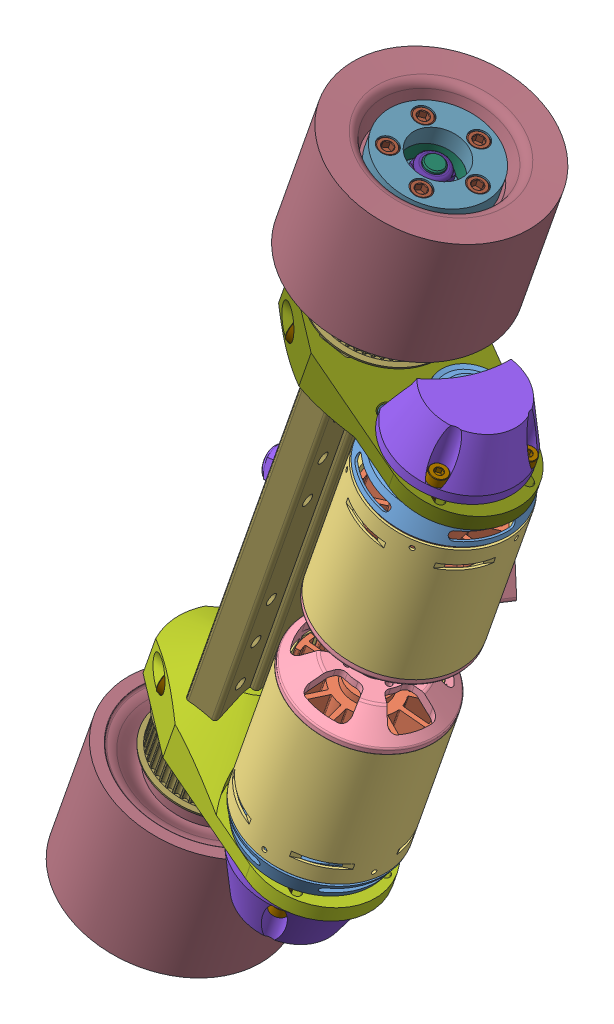
SolidWorks assembly MBS trucks pivot left, configuration Default. Lengths in mm.
Overall size (272 368.32 271.32).
89 component instances, 34 part files, 94 mates.
Components (placement in the parent):
- GPA26GT3150-A-N8-2: GPA26GT3150-A-N8 [Default] at (-15.9728 -53.3118 -54.0889) x (0.321551 0.946793 -0.013731) z (0.725283 -0.255593 -0.639248) size (20 28 28)
  - GPA26GT3150-A-N8_b-1: GPA26GT3150-A-N8_b [Default] at origin size (20 28 28)
  - SET-SCREW4-3-1: SET-SCREW4-3 [Default] at (10 5.4 0) x (0 -1 0) z (-1 0 0) size (3 4 4)
  - SET-SCREW4-3-2: SET-SCREW4-3 [Default] at (10 -2.2723 -3.2919) x (0 0.568065 0.822984) z (-1 0 0) size (3 4 4)
- Key20mm-2: Key20mm [Default] at (-13.4239 -54.1646 -53.2025) x (-0.725283 0.255593 0.639248) z (-0.608745 0.195591 -0.768878) size (3 20 3)
- MarkIITrucksCustomHanger pivot left-1: MarkIITrucksCustomHanger pivot left [Default] at (-31.1638 36.2817 -181.4556) x (-0.019038 0.999391 0.029249) z (0.838104 0 0.54551) size (362.13 183.87 195.64)
  - 50cal_baseplateEDIT-1: 50cal_baseplateEDIT [Default] at (40.8754 28.4427 48.4148) size (55.88 41.6 78.53)
  - BS_bushing-1: BS_bushing [Default] at (40.8754 74.2758 55.8381) x (0.903515 -0.328294 -0.275471) z (-0.428557 -0.692132 -0.580768) size (24.64 14.73 24.64)
  - BS_washer-1: BS_washer [Default] at (40.8754 63.8267 68.2909) x (0.781233 0.478195 0.401253) z (-0.624239 0.59846 0.502167) size (29.08 4.06 29.08)
  - kingpin-1: kingpin [Default] at (40.8754 51.905 82.4986) x (0.057682 0.764769 0.641717) z (0.998335 -0.044187 -0.037077) size (16.06 70.1 13.91)
  - kingpin-nut-1: kingpin-nut [90630A115] at (40.8754 87.1097 40.5433) x (0.976709 0.16437 0.137923) z (-0.214569 0.748202 0.627816) size (12.7 8.97 14.66)
  - Pivot_cup-1: Pivot_cup [Default] at (40.8754 44.9216 26.2393) x (-0.987309 0.102082 -0.121656) z (0.158811 0.63463 -0.756323) size (17.46 19.05 17.46)
  - RS_bushing-1: RS_bushing [Default] at (40.8754 76.7422 52.8988) x (0.999722 0.018072 0.015164) z (-0.023591 0.765831 0.642609) size (24.77 14.61 24.77)
  - washer-1: washer [Default] at (163.5053 59.317 96.5836) x (0.259291 0.957472 -0.126552) z (-0.223038 0.186855 0.956734) size (11 1 11)
  - BS_washer-2: BS_washer [Default] at (40.8754 87.1097 40.5433) x (-0.947616 0.244683 0.205314) z (0.319411 0.725916 0.609116) size (29.08 4.06 29.08)
  - washer-2: washer [Default] at (187.2325 53.7659 103.1992) x (-0.339774 -0.687707 0.641571) z (0.039134 -0.691901 -0.720931) size (11 1 11)
  - CustomHanger-1: CustomHanger [Default] at (40.8754 81.1126 56.6072) x (0.939693 -0.219846 0.262003) z (-0.34202 -0.604023 0.719846) size (253 93.96 18)
  - KegelWheelAssembly-1: KegelWheelAssembly [Default] at (219.4634 92.3673 64.2784) x (0.321079 0.830973 -0.454305) z (-0.11784 0.51103 0.851447) size (80 56 80)
    - Kegel 80mm longboard wheel-1: Kegel 80mm longboard wheel [Default] at (-60.1073 30.6906 17.2106) size (80 56 80)
    - 608-bearing-1: 608-bearing [6661K82] at (-60.1073 32.8534 17.2106) x (1 0 0) z (0 -1 0) size (22 22 7)
    - 608-bearing-2: 608-bearing [6661K82] at (-60.1073 15.6034 17.2106) x (-0.561464 0 0.827501) z (0 -1 0) size (22 22 7)
  - FPSSFJAD-D10-L64-T36-Q8-1: FPSSFJAD-D10-L64-T36-Q8 [Default] at (102.8951 73.4971 79.6845) x (0.939693 -0.219846 0.262003) z (-0.305917 -0.197698 0.931306) size (100 10 10)
  - SetScrew_SAE_10-32x.5in-1: SetScrew_SAE_10-32x.5in [92313A829] at (125.4477 77.0833 93.4091) x (0.758718 0.418725 -0.499016) z (0 0.766044 0.642788) size (4.96 4.83 13.07)
  - SetScrew_SAE_10-32x.5in-3: SetScrew_SAE_10-32x.5in [92313A829] at (125.446 59.3596 78.5344) x (0.758718 0.418725 -0.499016) z (0 -0.766044 -0.642788) size (4.96 4.83 13.07)
  - NylonLockNut_5.16-24-1: NylonLockNut_5.16-24 [97135A225] at (187.7024 53.656 103.3302) x (-0.176745 0.34369 0.922301) z (0.292812 0.912987 -0.284106) size (12.7 8.97 14.66)
  - KegelWheelAssembly-3: KegelWheelAssembly [Default] at (-99.1143 183.5416 5.8922) x (0.321079 0.830973 -0.454305) z (0.11784 -0.51103 -0.851447) size (80 56 80)
    - Kegel 80mm longboard wheel-1: Kegel 80mm longboard wheel [Default] at (-60.1073 30.6906 17.2106) size (80 56 80)
    - 608-bearing-1: 608-bearing [6661K82] at (-60.1073 32.8534 17.2106) x (1 0 0) z (0 -1 0) size (22 22 7)
    - 608-bearing-2: 608-bearing [6661K82] at (-60.1073 15.6034 17.2106) x (-0.561464 0 0.827501) z (0 -1 0) size (22 22 7)
  - FPSSFJAD-D10-L64-T36-Q8-3: FPSSFJAD-D10-L64-T36-Q8 [Default] at (-21.1443 102.5168 45.1001) x (-0.939693 0.219846 -0.262003) z (0.305917 0.197698 -0.931306) size (100 10 10)
  - NylonLockNut_5.16-24-3: NylonLockNut_5.16-24 [97135A225] at (-105.9516 122.3579 21.4544) x (0.176745 -0.34369 -0.922301) z (0.292812 0.912987 -0.284106) size (12.7 8.97 14.66)
  - SetScrew_SAE_10-32x.5in-7: SetScrew_SAE_10-32x.5in [92313A829] at (-43.6943 116.656 46.2483) x (-0.162487 0.634245 -0.755864) z (0 0.766044 0.642788) size (4.96 4.83 13.07)
  - SetScrew_SAE_10-32x.5in-8: SetScrew_SAE_10-32x.5in [92313A829] at (-43.6969 98.9306 31.3755) x (-0.162487 0.634245 -0.755864) z (0 -0.766044 -0.642788) size (4.96 4.83 13.07)
- 91274A172_COATED ALLOY STEEL SOCKET HEAD CAP SCREW-1: 91274A172_COATED ALLOY STEEL SOCKET HEAD CAP SCREW [91274A172] at (-39.3622 -9.9181 -56.7129) x (0.098878 -0.091252 0.990907) z (0.939117 -0.320732 -0.123247) size (9.53 9.53 32.48)
- 91274A172_COATED ALLOY STEEL SOCKET HEAD CAP SCREW-2: 91274A172_COATED ALLOY STEEL SOCKET HEAD CAP SCREW [91274A172] at (-43.3582 -9.0359 -89.4581) x (-0.342421 -0.903267 -0.258565) z (0.939117 -0.320732 -0.123247) size (9.53 9.53 32.48)
- 91274A172_COATED ALLOY STEEL SOCKET HEAD CAP SCREW-7: 91274A172_COATED ALLOY STEEL SOCKET HEAD CAP SCREW [91274A172] at (14.3369 148.1963 -59.006) x (-0.142744 -0.037907 -0.989034) z (0.939117 -0.320732 -0.123247) size (9.53 9.53 32.48)
- Turnigy6374-6: Turnigy6374 [Default] at (-10.4314 -14.5152 -52.975) x (0.287141 -0.111317 -0.951398) z (-0.902306 0.30198 -0.307657) size (83.4 113.65 83.4)
  - Stator-1: Stator [Default] at (3.7873 1.8989 -6.3731) size (58.75 9.22 58.75)
  - StatorPart2-1: StatorPart2 [Default] at (3.7873 -16.3511 -6.3731) size (50 66 50)
  - AxelHoldCover-1: AxelHoldCover [Default] at (3.7873 -60.8511 -6.3731) x (0.982235 0 -0.187653) z (0.187653 0 0.982235) size (59.15 61.5 59.15)
  - AxelHold-1: AxelHold [Default] at (3.7873 -60.8511 -6.3731) x (0.729158 0 0.684345) z (0.684345 0 -0.729158) size (59 18.5 59)
  - AxisCust-1: AxisCust [Default] at (3.7873 -73.3511 -6.3731) x (0.844889 0 -0.534942) z (0.534942 0 0.844889) size (8 113.65 8)
  - 90967A120_STAINLESS STEEL EXTERNAL RETAINING RING-1: 90967A120_STAINLESS STEEL EXTERNAL RETAINING RING [90967A120] at (3.7873 12.2489 -6.3731) x (0 -1 0) z (0 0 1) size (0.8 12.1 9.85)
  - 90967A120_STAINLESS STEEL EXTERNAL RETAINING RING-2: 90967A120_STAINLESS STEEL EXTERNAL RETAINING RING [90967A120] at (3.7873 -73.7511 -6.3731) x (0 -1 0) z (-0.841191 0 -0.540738) size (0.8 12.1 9.85)
- MotorMountLeft-3: MotorMountLeft [Default] at (-58.499 -16.8313 -71.1921) x (0.321551 0.946793 -0.013731) z (-0.287141 0.111317 0.951398) size (25.4 116.05 69.01)
- Belt Cap Wheel Side - Motor-2: Belt Cap Wheel Side - Motor [Default] at (-9.188 -33.3345 -54.3787) x (-0.287141 0.111317 0.951398) z (0.902306 -0.30198 0.307657) size (50.8 25 40.64)
- M4x16mm_BlackZincSteel-3: M4x16mm_BlackZincSteel [91274A119] at (13.174 -28.4024 -64.5577) x (0.938743 -0.320649 -0.126274) z (0.321551 0.946793 -0.013731) size (7 7 20.35)
- M4x16mm_BlackZincSteel-4: M4x16mm_BlackZincSteel [91274A119] at (4.2403 -24.939 -34.9571) x (0.938743 -0.320649 -0.126274) z (0.321551 0.946793 -0.013731) size (7 7 20.35)
- 92125A192_TYPE 18-8 SS FLAT-HEAD SOCKET CAP SCREW-9: 92125A192_TYPE 18-8 SS FLAT-HEAD SOCKET CAP SCREW [92125A192] at (-18.6935 -30.1791 -73.9677) x (-0.475481 0.17399 0.862349) z (-0.321551 -0.946793 0.013731) size (8 8 12.4)
- 92125A192_TYPE 18-8 SS FLAT-HEAD SOCKET CAP SCREW-10: 92125A192_TYPE 18-8 SS FLAT-HEAD SOCKET CAP SCREW [92125A192] at (-27.6272 -26.7157 -44.3671) x (0.938569 -0.320609 -0.127663) z (-0.321551 -0.946793 0.013731) size (8 8 12.4)
- 91251A355_BLACK-OXIDE ALLOY STEEL SOCKET HEAD CAP SCREW-11: 91251A355_BLACK-OXIDE ALLOY STEEL SOCKET HEAD CAP SCREW [91251A355] at (-57.9016 -22.5836 -86.7863) x (0.946372 -0.32086 0.0378) z (0.321551 0.946793 -0.013731) size (7.92 7.92 68.91)
- GPA50GT3150-A-H26_b-1: GPA50GT3150-A-H26_b [Default] at (-58.901 -18.0147 -71.1749) x (-0.321551 -0.946793 0.013731) z (0.936494 -0.315843 0.152386) size (20 51 51)
- Wheel Spacer 2-3: Wheel Spacer 2 [Default] at (-71.5742 -55.3305 -70.6337) x (-0.156301 0.038769 -0.986948) z (0.933903 -0.3195 -0.160451) size (44 14.02 44)
- Wheel Spacer Alum-3: Wheel Spacer Alum [Default] at (-71.5742 -55.3305 -70.6337) x (-0.156301 0.038769 -0.986948) z (0.933903 -0.3195 -0.160451) size (44 7.62 44)
- 91251A355_BLACK-OXIDE ALLOY STEEL SOCKET HEAD CAP SCREW-12: 91251A355_BLACK-OXIDE ALLOY STEEL SOCKET HEAD CAP SCREW [91251A355] at (-73.5512 -17.145 -78.2602) x (0.322292 -0.12307 -0.938606) z (0.321551 0.946793 -0.013731) size (7.92 7.92 68.91)
- 91251A355_BLACK-OXIDE ALLOY STEEL SOCKET HEAD CAP SCREW-13: 91251A355_BLACK-OXIDE ALLOY STEEL SOCKET HEAD CAP SCREW [91251A355] at (-70.6389 -17.8674 -59.8706) x (-0.747185 0.244798 -0.61789) z (0.321551 0.946793 -0.013731) size (7.92 7.92 68.91)
- 91251A355_BLACK-OXIDE ALLOY STEEL SOCKET HEAD CAP SCREW-14: 91251A355_BLACK-OXIDE ALLOY STEEL SOCKET HEAD CAP SCREW [91251A355] at (-53.1894 -23.7524 -57.0313) x (-0.784077 0.274364 0.556729) z (0.321551 0.946793 -0.013731) size (7.92 7.92 68.91)
- 91251A355_BLACK-OXIDE ALLOY STEEL SOCKET HEAD CAP SCREW-15: 91251A355_BLACK-OXIDE ALLOY STEEL SOCKET HEAD CAP SCREW [91251A355] at (-45.3173 -26.6672 -73.666) x (0.262598 -0.075232 0.961968) z (0.321551 0.946793 -0.013731) size (7.92 7.92 68.91)
- Wheel Spacer-3: Wheel Spacer [Default] at (-71.5742 -55.3305 -70.6337) x (0.139941 -0.061859 -0.988226) z (0.936494 -0.315843 0.152386) size (44 7.02 44)
- 91274A172_COATED ALLOY STEEL SOCKET HEAD CAP SCREW-8: 91274A172_COATED ALLOY STEEL SOCKET HEAD CAP SCREW [91274A172] at (14.3369 148.1963 -59.006) x (-0.142744 -0.037907 -0.989034) z (0.939117 -0.320732 -0.123247) size (9.53 9.53 32.48)
- 91274A172_COATED ALLOY STEEL SOCKET HEAD CAP SCREW-9: 91274A172_COATED ALLOY STEEL SOCKET HEAD CAP SCREW [91274A172] at (10.3408 149.0785 -91.7513) x (-0.27609 -0.917912 0.284977) z (0.939117 -0.320732 -0.123247) size (9.53 9.53 32.48)
- Turnigy6374-7: Turnigy6374 [Default] at (51.6181 130.4737 -51.2122) x (0.287141 -0.111317 -0.951398) z (0.902306 -0.30198 0.307657) size (83.4 113.65 83.4)
  - Stator-1: Stator [Default] at (3.7873 1.8989 -6.3731) size (58.75 9.22 58.75)
  - StatorPart2-1: StatorPart2 [Default] at (3.7873 -16.3511 -6.3731) size (50 66 50)
  - AxelHoldCover-1: AxelHoldCover [Default] at (3.7873 -60.8511 -6.3731) x (0.982235 0 -0.187653) z (0.187653 0 0.982235) size (59.15 61.5 59.15)
  - AxelHold-1: AxelHold [Default] at (3.7873 -60.8511 -6.3731) x (0.729158 0 0.684345) z (0.684345 0 -0.729158) size (59 18.5 59)
  - AxisCust-1: AxisCust [Default] at (3.7873 -73.3511 -6.3731) x (0.844889 0 -0.534942) z (0.534942 0 0.844889) size (8 113.65 8)
  - 90967A120_STAINLESS STEEL EXTERNAL RETAINING RING-1: 90967A120_STAINLESS STEEL EXTERNAL RETAINING RING [90967A120] at (3.7873 12.2489 -6.3731) x (0 -1 0) z (0 0 1) size (0.8 12.1 9.85)
  - 90967A120_STAINLESS STEEL EXTERNAL RETAINING RING-2: 90967A120_STAINLESS STEEL EXTERNAL RETAINING RING [90967A120] at (3.7873 -73.7511 -6.3731) x (0 -1 0) z (-0.841191 0 -0.540738) size (0.8 12.1 9.85)
- Belt Cap Wheel Side - Motor-3: Belt Cap Wheel Side - Motor [Default] at (52.5497 148.4497 -57.0151) x (0.287141 -0.111317 -0.951398) z (0.902306 -0.30198 0.307657) size (50.8 25 40.64)
- M4x16mm_BlackZincSteel-5: M4x16mm_BlackZincSteel [91274A119] at (67.1946 130.6588 -66.8646) x (0.938743 -0.320649 -0.126274) z (-0.321551 -0.946793 0.013731) size (7 7 20.35)
- M4x16mm_BlackZincSteel-6: M4x16mm_BlackZincSteel [91274A119] at (58.2608 134.1222 -37.264) x (0.938743 -0.320649 -0.126274) z (-0.321551 -0.946793 0.013731) size (7 7 20.35)
- 92125A192_TYPE 18-8 SS FLAT-HEAD SOCKET CAP SCREW-11: 92125A192_TYPE 18-8 SS FLAT-HEAD SOCKET CAP SCREW [92125A192] at (42.9157 151.2264 -76.5987) x (0.475481 -0.17399 -0.862349) z (0.321551 0.946793 -0.013731) size (8 8 12.4)
- 92125A192_TYPE 18-8 SS FLAT-HEAD SOCKET CAP SCREW-12: 92125A192_TYPE 18-8 SS FLAT-HEAD SOCKET CAP SCREW [92125A192] at (33.982 154.6898 -46.9981) x (0.938569 -0.320609 -0.127663) z (0.321551 0.946793 -0.013731) size (8 8 12.4)
- 91251A355_BLACK-OXIDE ALLOY STEEL SOCKET HEAD CAP SCREW-16: 91251A355_BLACK-OXIDE ALLOY STEEL SOCKET HEAD CAP SCREW [91251A355] at (7.0774 168.7443 -89.5611) x (0.946372 -0.32086 0.0378) z (-0.321551 -0.946793 0.013731) size (7.92 7.92 68.91)
- GPA50GT3150-A-H26_b-2: GPA50GT3150-A-H26_b [Default] at (3.6407 166.1364 -73.8457) x (0.321551 0.946793 -0.013731) z (-0.936494 0.315843 -0.152386) size (20 51 51)
- Wheel Spacer 2-4: Wheel Spacer 2 [Default] at (16.3139 203.4522 -74.3869) x (0.156301 -0.038769 0.986948) z (0.933903 -0.3195 -0.160451) size (44 14.02 44)
- Wheel Spacer Alum-4: Wheel Spacer Alum [Default] at (16.3139 203.4522 -74.3869) x (0.156301 -0.038769 0.986948) z (0.933903 -0.3195 -0.160451) size (44 7.62 44)
- Wheel Spacer-4: Wheel Spacer [Default] at (16.3139 203.4522 -74.3869) x (0.139941 -0.061859 -0.988226) z (-0.936494 0.315843 -0.152386) size (44 7.02 44)
- GPA26GT3150-A-N8-3: GPA26GT3150-A-N8 [Default] at (52.9034 149.4912 -57.0302) x (0.321551 0.946793 -0.013731) z (0.725283 -0.255593 -0.639248) size (20 28 28)
  - GPA26GT3150-A-N8_b-1: GPA26GT3150-A-N8_b [Default] at origin size (20 28 28)
  - SET-SCREW4-3-1: SET-SCREW4-3 [Default] at (10 5.4 0) x (0 -1 0) z (-1 0 0) size (3 4 4)
  - SET-SCREW4-3-2: SET-SCREW4-3 [Default] at (10 -2.2723 -3.2919) x (0 0.568065 0.822984) z (-1 0 0) size (3 4 4)
- Key20mm-3: Key20mm [Default] at (63.7096 166.9875 -54.1118) x (-0.725283 0.255593 0.639248) z (0.608745 -0.195591 0.768878) size (3 20 3)
- MotorMountRight-2: MotorMountRight [Default] at (3.2387 164.9529 -73.8285) x (0.321551 0.946793 -0.013731) z (-0.287141 0.111317 0.951398) size (25.4 116.05 69.01)
- 91251A355_BLACK-OXIDE ALLOY STEEL SOCKET HEAD CAP SCREW-17: 91251A355_BLACK-OXIDE ALLOY STEEL SOCKET HEAD CAP SCREW [91251A355] at (19.6617 164.6607 -76.4409) x (-0.262598 0.075232 -0.961968) z (-0.321551 -0.946793 0.013731) size (7.92 7.92 68.91)
- 91251A355_BLACK-OXIDE ALLOY STEEL SOCKET HEAD CAP SCREW-18: 91251A355_BLACK-OXIDE ALLOY STEEL SOCKET HEAD CAP SCREW [91251A355] at (11.7897 167.5755 -59.8061) x (-0.784077 0.274364 0.556729) z (-0.321551 -0.946793 0.013731) size (7.92 7.92 68.91)
- 91251A355_BLACK-OXIDE ALLOY STEEL SOCKET HEAD CAP SCREW-19: 91251A355_BLACK-OXIDE ALLOY STEEL SOCKET HEAD CAP SCREW [91251A355] at (-5.6598 173.4605 -62.6455) x (-0.747185 0.244798 -0.61789) z (-0.321551 -0.946793 0.013731) size (7.92 7.92 68.91)
- 91251A355_BLACK-OXIDE ALLOY STEEL SOCKET HEAD CAP SCREW-20: 91251A355_BLACK-OXIDE ALLOY STEEL SOCKET HEAD CAP SCREW [91251A355] at (-8.5722 174.1829 -81.0351) x (-0.322292 0.12307 0.938606) z (-0.321551 -0.946793 0.013731) size (7.92 7.92 68.91)
Mates (geometry in assembly coordinates):
- Concentric1: concentric anti-aligned: cylinder of ? through (0 89.5 0) axis (0 -1 0) radius 6; cylinder of ? through (0 92.55 0) axis (0 1 0) radius 6
- Concentric2: concentric anti-aligned: cylinder of ? through (0 -26.5 0) axis (0 1 0) radius 4; cylinder of GPA26GT3150-A-N8-2/GPA26GT3150-A-N8_b-1 through (0 -6.5 0) axis (0 -1 0) radius 4
- Coincident1: coincident aligned: plane of ? through (0 -26.5 0) normal (0 -1 0); plane of GPA26GT3150-A-N8-2/GPA26GT3150-A-N8_b-1 through (0 -26.5 0) normal (0 -1 0)
- Coincident7: coincident anti-aligned: line of ? through (-1.5 -26.5 -2.5) axis (0 0 -1); line of GPA26GT3150-A-N8-2/GPA26GT3150-A-N8_b-1 through (-1.5 -26.5 -5.4) axis (0 0 1)
- Coincident8: coincident aligned: plane of GPA26GT3150-A-N8-2/GPA26GT3150-A-N8_b-1 through (-15.9728 -53.3118 -54.0889) normal (-0.321551 -0.946793 0.013731); plane of Key20mm-2 through (-13.4239 -54.1646 -53.2025) normal (-0.321551 -0.946793 0.013731)
- Coincident9: coincident anti-aligned: plane of ? through (1.5 -6.5 -2.5) normal (0 0 -1); plane of Key20mm-2 through (-1.5 -6.5 -2.5) normal (0 0 1)
- Coincident10: coincident anti-aligned: plane of GPA26GT3150-A-N8-2/GPA26GT3150-A-N8_b-1 through (-5.1666 -35.8155 -51.1705) normal (-0.725283 0.255593 0.639248); plane of Key20mm-2 through (-6.9928 -35.2288 -53.4771) normal (0.725283 -0.255593 -0.639248)
- Concentric5: concentric anti-aligned: cylinder of MarkIITrucksCustomHanger pivot left-1/CustomHanger-1 through (-77.4086 -5.45 -20.7444) axis (0 -1 0) radius 9; cylinder of ? through (-77.4086 -27.45 -20.7444) axis (0 1 0) radius 11
- Coincident15: coincident anti-aligned: plane of ? through (-77.2299 -26.5 -21.3999) normal (0 1 0); plane of ? through (-51.5162 -26.5 -25.2476) normal (0 -1 0)
- Coincident28: coincident anti-aligned: plane of MarkIITrucksCustomHanger pivot left-1/CustomHanger-1; plane of ? through (-34.0921 -14.7886 -63.0299) normal (-0.017088 0 -0.999854)
- Coincident37: coincident aligned: plane of ? through (-44.2534 59.243 -27.1128) normal (-0.40707 0 0.913397); plane of ? through (38.0802 32.893 9.5804) normal (-0.40707 0 0.913397)
- Coincident38: coincident anti-aligned: plane of ? through (-30.006 52.893 -59.0817) normal (0 -1 0); plane of ? through (52.3276 52.893 -22.3885) normal (0 1 0)
- Coincident40: coincident anti-aligned: plane of ? through (0 0 0) normal (0 -1 0); plane of ? through (-73.3266 0 -32.3363) normal (0 1 0)
- Concentric12: concentric aligned: cylinder of ? through (0 -26.5 0) axis (0 1 0) radius 4; cylinder of ? through (0 -6.35 0) axis (0 1 0) radius 6
- Coincident41: coincident anti-aligned: plane of ?; plane of ? through (-51.7284 -27.45 -24.8099) normal (0 -1 0)
- Concentric17: concentric aligned: cylinder of MarkIITrucksCustomHanger pivot left-1/CustomHanger-1 through (-34.2459 -20.2386 -72.0286) axis (0 -1 0) radius 9; cylinder of ? through (-34.2459 -22.2386 -72.0286) axis (0 -1 0) radius 10
- Coincident43: coincident anti-aligned: plane of ?; plane of ? through (-34.2459 -42.2386 -72.0286) normal (0 -1 0)
- Concentric18: concentric anti-aligned: cylinder of ? through (-93.4436 208.55 -19.2392) axis (0 -1 0) radius 2.54; cylinder of ? through (-93.4436 193.63 -19.2392) axis (0 1 0) radius 2.413
- Coincident45: coincident anti-aligned: plane of ? through (-93.4436 193.63 -19.2392) normal (0 -1 0); plane of ? through (-93.4436 193.63 -19.2392) normal (0 1 0)
- Concentric19: concentric: cylinder of ? through (-93.4436 208.55 -19.2392) axis (0 -1 0) radius 2.54; cylinder of ? through (-93.4436 193.63 -19.2392) axis (0 1 0) radius 2.413
- Coincident47: coincident anti-aligned: plane of ? through (-93.4436 193.63 -19.2392) normal (0 -1 0); plane of ? through (-93.4436 193.63 -19.2392) normal (0 1 0)
- Coincident48: coincident anti-aligned: plane of ?; plane of ? through (-43.0816 192.3928 -91.4524) normal (-0.019038 0.999391 0.029249)
- Concentric28: concentric anti-aligned: cylinder of ? through (-15.3407 192.0809 -62.7407) axis (-0.019038 0.999391 0.029249) radius 2.9; cylinder of ? through (-16.2508 239.8547 -61.3425) axis (0.019038 -0.999391 -0.029249) radius 2.413
- Coincident56: coincident anti-aligned: plane of GPA26GT3150-A-N8-2/GPA26GT3150-A-N8_b-1 through (-7.3425 -35.0487 -49.2527) normal (-0.608745 0.195591 -0.768878); plane of Key20mm-2 through (-5.1666 -35.8155 -51.1705) normal (0.608745 -0.195591 0.768878)
- Coincident58: coincident aligned: plane of GPA26GT3150-A-N8-2/GPA26GT3150-A-N8_b-1; plane of ? through (-22.9313 -22.2386 -48.6196) normal (0 1 0)
- Concentric38: concentric aligned: cylinder of MarkIITrucksCustomHanger pivot left-1/CustomHanger-1 through (-41.8828 -7.7386 -55.3957) axis (0.999854 0 -0.017088) radius 2.3813; cylinder of ? through (-80.4696 -7.7386 -54.7362) axis (0.999854 0 -0.017088) radius 5
- Concentric40: concentric aligned: cylinder of ? through (-81.0335 -7.7386 -87.7314) axis (0.999854 0 -0.017088) radius 5; cylinder of 91274A172_COATED ALLOY STEEL SOCKET HEAD CAP SCREW-2 through (-52.2253 -7.7386 -88.2237) axis (0.999854 0 -0.017088) radius 4.7625
- Concentric41: concentric aligned: cylinder of ? through (-80.4696 -7.7386 -54.7362) axis (0.999854 0 -0.017088) radius 5; cylinder of 91274A172_COATED ALLOY STEEL SOCKET HEAD CAP SCREW-1 through (-51.6614 -7.7386 -55.2286) axis (0.999854 0 -0.017088) radius 4.7625
- Coincident61: coincident anti-aligned: plane of ? through (-45.3123 -7.7386 -55.3371) normal (-0.999854 0 0.017088); plane of 91274A172_COATED ALLOY STEEL SOCKET HEAD CAP SCREW-1 through (-45.3123 -7.7386 -55.3371) normal (0.999854 0 -0.017088)
- Coincident62: coincident anti-aligned: plane of ? through (-45.8762 -7.7386 -88.3322) normal (-0.999854 0 0.017088); plane of 91274A172_COATED ALLOY STEEL SOCKET HEAD CAP SCREW-2 through (-45.8762 -7.7386 -88.3322) normal (0.999854 0 -0.017088)
- Coincident65: coincident anti-aligned: plane of MarkIITrucksCustomHanger pivot left-1/CustomHanger-1; plane of ? through (-40.595 4.2614 -71.9201) normal (0.999854 0 -0.017088)
- Coincident68: coincident anti-aligned: plane of ? through (-34.2459 -14.7886 -72.0286) normal (0 1 0); plane of Turnigy6374-6/Stator-1 through (52.6547 -14.7886 -33.3) normal (0 -1 0)
- Concentric46: concentric anti-aligned: cylinder of GPA26GT3150-A-N8-2/GPA26GT3150-A-N8_b-1 through (-9.5418 -34.3759 -54.3635) axis (-0.321551 -0.946793 0.013731) radius 4; cylinder of Turnigy6374-6/AxisCust-1 through (-15.6995 -52.507 -54.1006) axis (0.321551 0.946793 -0.013731) radius 4
- Coincident70: coincident anti-aligned: plane of Key20mm-2 through (-6.9928 -35.2288 -53.4771) normal (0.725283 -0.255593 -0.639248); plane of Turnigy6374-6/AxisCust-1 through (-5.1057 -35.8351 -51.0936) normal (-0.725283 0.255593 0.639248)
- Concentric55: concentric aligned: cylinder of 91274A172_COATED ALLOY STEEL SOCKET HEAD CAP SCREW-1 through (-51.6614 -7.7386 -55.2286) axis (0.999854 0 -0.017088) radius 4.7625; cylinder of ? through (-80.4696 -7.7386 -54.7362) axis (0.999854 0 -0.017088) radius 3.175
- Coincident75: coincident anti-aligned: plane of 91274A172_COATED ALLOY STEEL SOCKET HEAD CAP SCREW-1; plane of ? through (-45.3123 -7.7386 -55.3371) normal (-0.999854 0 0.017088)
- Coincident76: coincident anti-aligned: plane of MarkIITrucksCustomHanger pivot left-1/CustomHanger-1; plane of ? through (-40.595 4.2614 -71.9201) normal (0.999854 0 -0.017088)
- Coincident77: coincident anti-aligned: plane of MarkIITrucksCustomHanger pivot left-1/CustomHanger-1; plane of ? through (-34.0921 -14.7886 -63.0299) normal (-0.017088 0 -0.999854)
- Concentric56: concentric aligned: cylinder of 91274A172_COATED ALLOY STEEL SOCKET HEAD CAP SCREW-2 through (-54.3819 -7.7386 -88.1869) axis (0.999854 0 -0.017088) radius 4.7625; cylinder of ? through (-81.0335 -7.7386 -87.7314) axis (0.999854 0 -0.017088) radius 5
- Concentric57: concentric aligned: cylinder of MarkIITrucksCustomHanger pivot left-1/CustomHanger-1 through (-41.8828 -7.7386 -55.3957) axis (0.999854 0 -0.017088) radius 2.3813; cylinder of ? through (-80.4696 -7.7386 -54.7362) axis (0.999854 0 -0.017088) radius 5
- Concentric58: concentric aligned: cylinder of 91274A172_COATED ALLOY STEEL SOCKET HEAD CAP SCREW-7 through (-51.6614 159.2614 -55.2286) axis (0.999854 0 -0.017088) radius 4.7625; cylinder of ? through (-80.4696 159.2614 -54.7362) axis (0.999854 0 -0.017088) radius 5
- Coincident78: coincident anti-aligned: plane of 91274A172_COATED ALLOY STEEL SOCKET HEAD CAP SCREW-7; plane of ? through (-45.3123 159.2614 -55.3371) normal (-0.999854 0 0.017088)
- Concentric59: concentric aligned: cylinder of 91274A172_COATED ALLOY STEEL SOCKET HEAD CAP SCREW-8 through (-52.2253 159.2614 -88.2237) axis (0.999854 0 -0.017088) radius 4.7625; cylinder of ? through (-81.0335 159.2614 -87.7314) axis (0.999854 0 -0.017088) radius 5
- Coincident79: coincident anti-aligned: plane of MarkIITrucksCustomHanger pivot left-1/CustomHanger-1; plane of ? through (-43.2446 -0.6886 -71.8748) normal (0.999854 0 -0.017088)
- Concentric60: concentric anti-aligned: cylinder of 91274A172_COATED ALLOY STEEL SOCKET HEAD CAP SCREW-2 through (-52.2253 -7.7386 -88.2237) axis (0.999854 0 -0.017088) radius 4.7625; circle of ?
- Coincident80: coincident anti-aligned: plane of 91274A172_COATED ALLOY STEEL SOCKET HEAD CAP SCREW-2; plane of ? through (-45.8762 -7.7386 -88.3322) normal (-0.999854 0 0.017088)
- Concentric61: concentric aligned: cylinder of MarkIITrucksCustomHanger pivot left-1/CustomHanger-1 through (-63.9155 -2.015 -86.7603) axis (0.939117 -0.320732 -0.123247) radius 2.3813; cylinder of 91274A172_COATED ALLOY STEEL SOCKET HEAD CAP SCREW-2 through (-73.1752 1.1474 -85.5451) axis (0.939117 -0.320732 -0.123247) radius 4.7625
- Concentric62: concentric aligned: cylinder of MarkIITrucksCustomHanger pivot left-1/CustomHanger-1 through (-41.8828 -7.7386 -55.3957) axis (0.999854 0 -0.017088) radius 2.3813; cylinder of ? through (-80.4696 -7.7386 -54.7362) axis (0.999854 0 -0.017088) radius 3.175
- Concentric63: concentric: cylinder of 91274A172_COATED ALLOY STEEL SOCKET HEAD CAP SCREW-1 through (-51.6614 -7.7386 -55.2286) axis (0.999854 0 -0.017088) radius 4.7625; cylinder of ? through (-80.4696 -7.7386 -54.7362) axis (0.999854 0 -0.017088) radius 5
- Coincident81: coincident anti-aligned: plane of 91274A172_COATED ALLOY STEEL SOCKET HEAD CAP SCREW-1; plane of ? through (-45.3123 -7.7386 -55.3371) normal (-0.999854 0 0.017088)
- Coincident86: coincident aligned: plane of GPA26GT3150-A-N8-2/GPA26GT3150-A-N8_b-1 through (-15.9728 -53.3118 -54.0889) normal (-0.321551 -0.946793 0.013731); plane of Turnigy6374-6/AxisCust-1 through (-15.9728 -53.3118 -54.0889) normal (-0.321551 -0.946793 0.013731)
- Coincident87: coincident anti-aligned: plane of MarkIITrucksCustomHanger pivot left-1/CustomHanger-1; plane of ? through (-33.8358 147.2614 -48.0321) normal (-0.017088 0 -0.999854)
- Concentric72: concentric aligned: cylinder of MarkIITrucksCustomHanger pivot left-1/CustomHanger-1 through (-6.2204 155.2171 -56.3081) axis (0.939117 -0.320732 -0.123247) radius 2.3813; cylinder of 91274A172_COATED ALLOY STEEL SOCKET HEAD CAP SCREW-7 through (-15.4801 158.3795 -55.0929) axis (0.939117 -0.320732 -0.123247) radius 4.7625
- Concentric73: concentric aligned: cylinder of 91274A172_COATED ALLOY STEEL SOCKET HEAD CAP SCREW-1 through (-69.1791 0.2651 -52.7998) axis (0.939117 -0.320732 -0.123247) radius 4.7625; cylinder of MotorMountLeft-3 through (-123.8058 18.9215 -45.6308) axis (0.939117 -0.320732 -0.123247) radius 5
- Concentric74: concentric aligned: cylinder of 91274A172_COATED ALLOY STEEL SOCKET HEAD CAP SCREW-2 through (-73.1752 1.1474 -85.5451) axis (0.939117 -0.320732 -0.123247) radius 4.7625; cylinder of MotorMountLeft-3 through (-127.8019 19.8037 -78.376) axis (0.939117 -0.320732 -0.123247) radius 5
- Coincident99: coincident anti-aligned: plane of MarkIITrucksCustomHanger pivot left-1/CustomHanger-1 through (4.6296 200.2711 -82.1167) normal (-0.939117 0.320732 0.123247); plane of MotorMountLeft-3 through (-64.9093 -7.9325 -70.1701) normal (0.939117 -0.320732 -0.123247)
- Coincident100: coincident anti-aligned: plane of 91274A172_COATED ALLOY STEEL SOCKET HEAD CAP SCREW-1 through (-63.2157 -1.7715 -53.5824) normal (0.939117 -0.320732 -0.123247); plane of MotorMountLeft-3 through (-63.2157 -1.7715 -53.5824) normal (-0.939117 0.320732 0.123247)
- Coincident101: coincident anti-aligned: plane of 91274A172_COATED ALLOY STEEL SOCKET HEAD CAP SCREW-2 through (-67.2118 -0.8893 -86.3277) normal (0.939117 -0.320732 -0.123247); plane of MotorMountLeft-3 through (-67.2118 -0.8893 -86.3277) normal (-0.939117 0.320732 0.123247)
- Coincident108: coincident anti-aligned: plane of Turnigy6374-6/Stator-1 through (-7.1462 -27.3223 -54.4658) normal (-0.321551 -0.946793 0.013731); plane of MotorMountLeft-3 through (-56.4572 -10.8191 -71.2793) normal (0.321551 0.946793 -0.013731)
- Concentric92: concentric aligned: cylinder of Belt Cap Wheel Side - Motor-2 through (0.9551 -64.3805 -64.0359) axis (0.321551 0.946793 -0.013731) radius 4; cylinder of M4x16mm_BlackZincSteel-3 through (6.743 -47.3382 -64.2831) axis (0.321551 0.946793 -0.013731) radius 3.5
- Concentric93: concentric aligned: cylinder of Belt Cap Wheel Side - Motor-2 through (-7.9786 -60.9171 -34.4353) axis (0.321551 0.946793 -0.013731) radius 4; cylinder of M4x16mm_BlackZincSteel-4 through (-2.1907 -43.8748 -34.6825) axis (0.321551 0.946793 -0.013731) radius 3.5
- Coincident121: coincident anti-aligned: plane of Belt Cap Wheel Side - Motor-2 through (8.0292 -43.551 -64.338) normal (-0.321551 -0.946793 0.013731); plane of M4x16mm_BlackZincSteel-3 through (8.0292 -43.551 -64.338) normal (0.321551 0.946793 -0.013731)
- Coincident122: coincident anti-aligned: plane of Belt Cap Wheel Side - Motor-2 through (-0.9045 -40.0877 -34.7374) normal (-0.321551 -0.946793 0.013731); plane of M4x16mm_BlackZincSteel-4 through (-0.9045 -40.0877 -34.7374) normal (0.321551 0.946793 -0.013731)
- Coincident123: coincident anti-aligned: plane of MotorMountLeft-3 through (-58.499 -16.8313 -71.1921) normal (-0.321551 -0.946793 0.013731); plane of Belt Cap Wheel Side - Motor-2 through (-9.188 -33.3345 -54.3787) normal (0.321551 0.946793 -0.013731)
- Tangent4: tangent anti-aligned: plane of MotorMountLeft-3; cone of ? through (71.8505 -7.1277 -46.5804) axis (-0.019038 0.999391 0.029249)
- Tangent5: tangent anti-aligned: plane of MotorMountLeft-3; cone of ? through (89.6321 -19.6632 -21.2486) axis (-0.019038 0.999391 0.029249)
- Tangent9: tangent anti-aligned: plane of MotorMountLeft-3; cone of ? through (89.6321 -19.6632 -21.2486) axis (-0.019038 0.999391 0.029249)
- Tangent10: tangent: plane of MotorMountLeft-3; curve of ?
- Concentric105: concentric anti-aligned: cylinder of Turnigy6374-6/Stator-1 through (89.3833 -6.6015 -20.8663) axis (0.019038 -0.999391 -0.029249) radius 1.8559; circle of ?
- Concentric106: concentric anti-aligned: cylinder of Turnigy6374-6/Stator-1 through (71.8325 -6.1841 -46.5528) axis (0.019038 -0.999391 -0.029249) radius 1.8559; circle of ?
- Concentric107: concentric anti-aligned: cylinder of Turnigy6374-6/Stator-1 through (14.3218 -25.0226 -64.6067) axis (-0.321551 -0.946793 0.013731) radius 1.8559; circle of M4x16mm_BlackZincSteel-3
- Concentric108: concentric anti-aligned: cylinder of Turnigy6374-6/Stator-1 through (5.3881 -21.5593 -35.0061) axis (-0.321551 -0.946793 0.013731) radius 1.8559; cylinder of M4x16mm_BlackZincSteel-4 through (-2.1907 -43.8748 -34.6825) axis (0.321551 0.946793 -0.013731) radius 3.5
- Tangent18: tangent anti-aligned: plane of MotorMountLeft-3 through (-52.7401 -19.0639 -90.2737) normal (-0.43041 -0.59077 0.68245); cone of 92125A192_TYPE 18-8 SS FLAT-HEAD SOCKET CAP SCREW-9 through (-17.9539 -28.0015 -73.9993) axis (0.321551 0.946793 -0.013731)
- Tangent19: tangent anti-aligned: plane of MotorMountLeft-3 through (-62.7363 -12.5099 -54.5233) normal (-0.024332 -0.748197 -0.663031); cone of 92125A192_TYPE 18-8 SS FLAT-HEAD SOCKET CAP SCREW-10 through (-26.8876 -24.5381 -44.3987) axis (0.321551 0.946793 -0.013731)
- Concentric109: concentric anti-aligned: cylinder of Turnigy6374-6/Stator-1 through (-22.6851 -12.1638 -44.5782) axis (-0.321551 -0.946793 0.013731) radius 1.8559; circle of 92125A192_TYPE 18-8 SS FLAT-HEAD SOCKET CAP SCREW-10
- Concentric110: concentric anti-aligned: cylinder of Turnigy6374-6/Stator-1 through (-13.7513 -15.6272 -74.1787) axis (-0.321551 -0.946793 0.013731) radius 1.8559; circle of 92125A192_TYPE 18-8 SS FLAT-HEAD SOCKET CAP SCREW-9
- Coincident124: coincident aligned: cone of MotorMountLeft-3 through (-26.8876 -24.5381 -44.3987) axis (0.321551 0.946793 -0.013731); cone of 92125A192_TYPE 18-8 SS FLAT-HEAD SOCKET CAP SCREW-10 through (-26.8876 -24.5381 -44.3987) axis (0.321551 0.946793 -0.013731)
- Coincident140: coincident anti-aligned: plane of ? through (-15.0116 238.8514 -69.4308) normal (0.019038 -0.999391 -0.029249); plane of ? through (-15.0116 238.8514 -69.4308) normal (-0.019038 0.999391 0.029249)
- Concentric122: concentric aligned: cylinder of MotorMountLeft-3 through (8.1417 -43.2197 -64.3428) axis (0.321551 0.946793 -0.013731) radius 2; cylinder of M4x16mm_BlackZincSteel-3 through (6.743 -47.3382 -64.2831) axis (0.321551 0.946793 -0.013731) radius 3.5
- Concentric128: concentric anti-aligned: cylinder of 91251A355_BLACK-OXIDE ALLOY STEEL SOCKET HEAD CAP SCREW-11 through (-79.8719 -87.2741 -85.848) axis (0.321551 0.946793 -0.013731) radius 3.9624; cylinder of Wheel Spacer Alum-3 through (-78.3201 -82.7049 -85.9143) axis (-0.321551 -0.946793 0.013731) radius 3.9688
- Coincident145: coincident anti-aligned: plane of 91251A355_BLACK-OXIDE ALLOY STEEL SOCKET HEAD CAP SCREW-11 through (-78.3201 -82.7049 -85.9143) normal (0.321551 0.946793 -0.013731); plane of Wheel Spacer Alum-3 through (-78.3201 -82.7049 -85.9143) normal (-0.321551 -0.946793 0.013731)
- Coincident146: coincident aligned: circle of MarkIITrucksCustomHanger pivot left-1/KegelWheelAssembly-3/Kegel 80mm longboard wheel-1; circle of Wheel Spacer-3
- Concentric129: concentric aligned: cylinder of MarkIITrucksCustomHanger pivot left-1/KegelWheelAssembly-3/Kegel 80mm longboard wheel-1 through (-76.0924 -33.925 -59.6378) axis (-0.321551 -0.946793 0.013731) radius 2.9; cylinder of Wheel Spacer-3 through (-87.9898 -68.9563 -59.1297) axis (-0.321551 -0.946793 0.013731) radius 2.54
- Coincident147: coincident anti-aligned: plane of Wheel Spacer Alum-3 through (-79.7214 -79.3196 -70.2858) normal (0.321551 0.946793 -0.013731); plane of Wheel Spacer-3 through (-79.7214 -79.3196 -70.2858) normal (-0.321551 -0.946793 0.013731)
- Concentric130: concentric aligned: circle of Wheel Spacer Alum-3; circle of Wheel Spacer-3
- Concentric131: concentric aligned: circle of Wheel Spacer Alum-3; circle of Wheel Spacer-3
- Concentric132: concentric aligned: cylinder of MarkIITrucksCustomHanger pivot left-1/KegelWheelAssembly-3/Kegel 80mm longboard wheel-1 through (-65.5732 -37.6607 -70.89) axis (0.321551 0.946793 -0.013731) radius 40; cylinder of GPA50GT3150-A-H26_b-1 through (-65.332 -36.9506 -70.9003) axis (0.321551 0.946793 -0.013731) radius 13
- Coincident148: coincident aligned: circle of MarkIITrucksCustomHanger pivot left-1/KegelWheelAssembly-3/Kegel 80mm longboard wheel-1; circle of Wheel Spacer 2-3
- Coincident149: coincident anti-aligned: plane of GPA50GT3150-A-H26_b-1 through (-62.3932 -38.2496 -91.653) normal (-0.321551 -0.946793 0.013731); plane of Wheel Spacer 2-3 through (-65.332 -36.9506 -70.9003) normal (0.321551 0.946793 -0.013731)
- Concentric133: concentric aligned: cylinder of Wheel Spacer 2-3 through (-83.2652 -45.7476 -77.8454) axis (0.321551 0.946793 -0.013731) radius 2.54; cylinder of 91251A355_BLACK-OXIDE ALLOY STEEL SOCKET HEAD CAP SCREW-12 through (-93.9697 -77.2663 -77.3883) axis (0.321551 0.946793 -0.013731) radius 2.413
- Concentric134: concentric aligned: cylinder of GPA50GT3150-A-H26_b-1 through (-78.7635 -32.4925 -78.0377) axis (0.321551 0.946793 -0.013731) radius 2; cylinder of 91251A355_BLACK-OXIDE ALLOY STEEL SOCKET HEAD CAP SCREW-12 through (-93.9697 -77.2663 -77.3883) axis (0.321551 0.946793 -0.013731) radius 2.413
- Coincident154: coincident aligned: plane of MarkIITrucksCustomHanger pivot left-1/CustomHanger-1 through (-3.8145 167.2302 -81.9765) normal (0.321551 0.946793 -0.013731); plane of MotorMountRight-2 through (3.2387 164.9529 -73.8285) normal (0.321551 0.946793 -0.013731)
- Coincident155: coincident anti-aligned: plane of MarkIITrucksCustomHanger pivot left-1/CustomHanger-1 through (21.5337 194.4979 -84.3352) normal (0.939117 -0.320732 -0.123247); plane of MotorMountRight-2 through (9.6489 156.0542 -74.8506) normal (-0.939117 0.320732 0.123247)
- Coincident156: coincident anti-aligned: plane of MarkIITrucksCustomHanger pivot left-1/CustomHanger-1 through (-30.6873 75.4559 -47.913) normal (0.121093 -0.026735 0.992281); plane of MotorMountRight-2 through (-2.0224 140.2628 -49.665) normal (-0.121093 0.026735 -0.992281)
